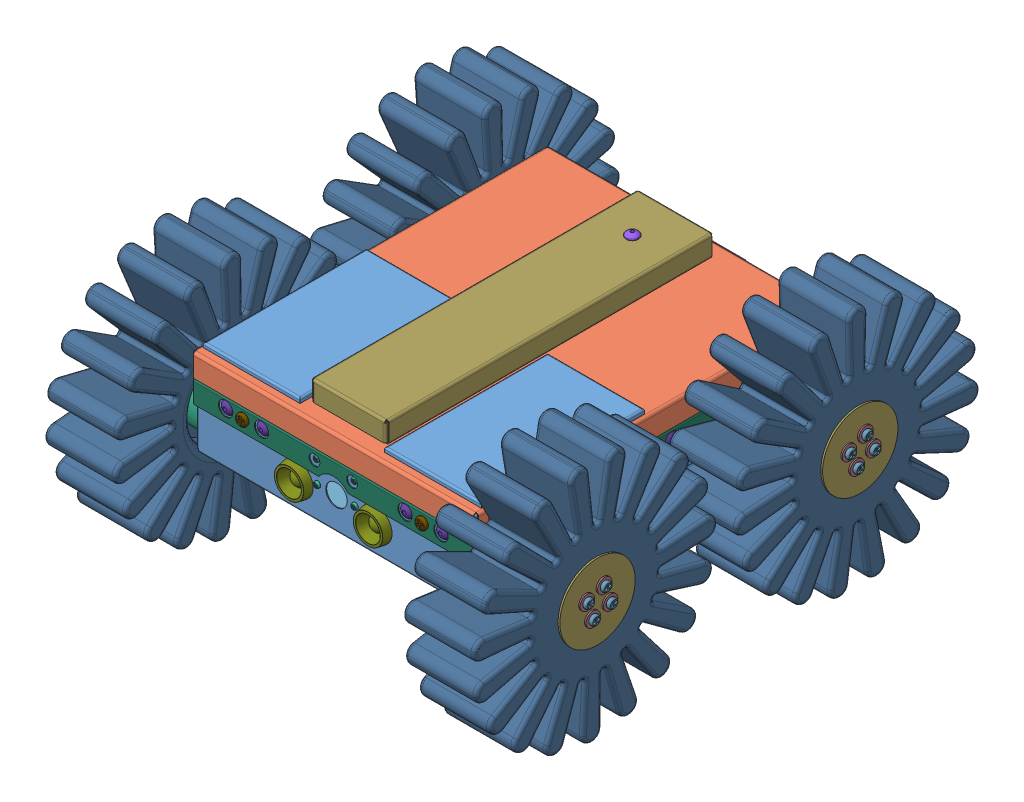
SolidWorks assembly GB0814, configuration Default. Lengths in mm.
Overall size (247.76 181.13 312.99).
487 component instances, 71 part files, 459 mates.
Components (placement in the parent):
- case.bottom-1: case.bottom [Default<As Machined>] at origin size (156 42.5 195.44)
- SM4315R-1: SM4315R [Default] at (47.1812 21 161.9111) x (0 -1 0) z (0 0 -1) size (20.32 45.78 53.29)
- SM4315R-2: SM4315R [Default] at (47.1812 21 17.796) x (0 1 0) z (0 0 1) size (20.32 45.78 53.29)
- SM4315R-3: SM4315R [Default] at (107.8188 21 17.796) x (0 -1 0) z (0 0 1) size (20.32 45.78 53.29)
- SM4315R-4: SM4315R [Default] at (107.8188 21 161.9111) x (0 1 0) z (0 0 -1) size (20.32 45.78 53.29)
- raspberrypi_b_+_(assembly)-1: raspberrypi_b_+_(assembly) [Valor predeterminado] at (78.9157 12.4 7.5062) x (0 0 -1) z (0 1 0) size (88.51 58.54 18.92)
  - raspberry_pi_B+_(bar_180_2x20)-1: raspberry_pi_B+_(bar_180_2x20) [Default] at (-150.8088 26.71 4.1) x (0 1 0) z (-1 0 0) size (5.08 11.6 50.8)
  - raspberry_pi_B+_(QFN64)-1: raspberry_pi_B+_(QFN64) [Default] at (-101.7896 6.9461 1.6) x (0 -1 0) z (-1 0 0) size (9.04 0.9 9.04)
  - raspberry_pi_B+_(168_FBGA_12x12)-1: raspberry_pi_B+_(168_FBGA_12x12) [Valor predeterminado] at (-129.6291 3.2481 1.87) size (12 12 0.71)
  - raspberry_pi_B+_(USB_x2)-1: raspberry_pi_B+_(USB_x2) [Valor predeterminado] at (-81.197 116.594 21.0675) x (0 1 0) z (1 0 0) size (14.7 17.85 17.4)
    - raspberry_pi_B+_(USB_x2_part1)-1: raspberry_pi_B+_(USB_x2_part1) [По умолчанию] at (-114.6616 -10.9375 -4.85) x (0 0 1) z (-1 0 0) size (17.4 6.35 14.7)
    - raspberry_pi_B+_(USB_x2_part2)-1: raspberry_pi_B+_(USB_x2_part2) [По умолчанию] at (-114.6616 -19.4375 -4.85) x (0 0 1) z (-1 0 0) size (17.4 11.5 14.7)
  - raspberry_pi_B+_(micro_USB)-1: raspberry_pi_B+_(micro_USB) [Default] at (-134.0345 -42.9478 -3.6369) x (1 0 0) z (0 -1 0) size (7.97 2.92 5.43)
    - raspberry_pi_B+_(micro_USB_cover)-1: raspberry_pi_B+_(micro_USB_cover) [Default] at (-14.4796 6.4719 -16.0085) size (7.97 2.92 5.43)
    - raspberry_pi_B+_(micro_USB_contacts)-1: raspberry_pi_B+_(micro_USB_contacts) [Default] at (-14.4796 6.4719 -20.7085) size (6.9 2.16 4.2)
  - raspberry_pi_B+_(HDMI_socket)-1: raspberry_pi_B+_(HDMI_socket) [Default] at (-127.1025 -18.8313 5.025) x (1 0 0) z (0 -1 0) size (16.2 8 9.9)
    - raspberry_pi__HDMI_socket_cover-1: raspberry_pi__HDMI_socket_cover [Default] at (-20 0 0) size (16.2 8 9)
    - raspberry_pi__HDMI_socket_inside-1: raspberry_pi__HDMI_socket_inside [Default] at (-20 0 0) size (15 6.1 7.6)
    - raspberry_pi__HDMI_socket_large_pin-1: raspberry_pi__HDMI_socket_large_pin [Valor predeterminado] at (-201.7661 0.45 76.5103) x (0 0 -1) z (0 -1 0) size (7.55 0.65 3.84)
    - raspberry_pi__HDMI_socket_small_pin-1: raspberry_pi__HDMI_socket_small_pin [Valor predeterminado] at (-202.2661 -0.25 76.5103) x (0 0 -1) z (0 -1 0) size (7.55 0.65 3.08)
    - raspberry_pi__HDMI_socket_large_pin-2: raspberry_pi__HDMI_socket_large_pin [Valor predeterminado] at (-202.7661 0.45 76.5103) x (0 0 -1) z (0 -1 0) size (7.55 0.65 3.84)
    - raspberry_pi__HDMI_socket_large_pin-3: raspberry_pi__HDMI_socket_large_pin [Valor predeterminado] at (-203.7661 0.45 76.5103) x (0 0 -1) z (0 -1 0) size (7.55 0.65 3.84)
    - raspberry_pi__HDMI_socket_large_pin-4: raspberry_pi__HDMI_socket_large_pin [Valor predeterminado] at (-204.7661 0.45 76.5103) x (0 0 -1) z (0 -1 0) size (7.55 0.65 3.84)
    - raspberry_pi__HDMI_socket_large_pin-5: raspberry_pi__HDMI_socket_large_pin [Valor predeterminado] at (-205.7661 0.45 76.5103) x (0 0 -1) z (0 -1 0) size (7.55 0.65 3.84)
    - raspberry_pi__HDMI_socket_large_pin-6: raspberry_pi__HDMI_socket_large_pin [Valor predeterminado] at (-206.7661 0.45 76.5103) x (0 0 -1) z (0 -1 0) size (7.55 0.65 3.84)
    - raspberry_pi__HDMI_socket_large_pin-7: raspberry_pi__HDMI_socket_large_pin [Valor predeterminado] at (-207.7661 0.45 76.5103) x (0 0 -1) z (0 -1 0) size (7.55 0.65 3.84)
    - raspberry_pi__HDMI_socket_large_pin-8: raspberry_pi__HDMI_socket_large_pin [Valor predeterminado] at (-208.7661 0.45 76.5103) x (0 0 -1) z (0 -1 0) size (7.55 0.65 3.84)
    - raspberry_pi__HDMI_socket_large_pin-9: raspberry_pi__HDMI_socket_large_pin [Valor predeterminado] at (-209.7661 0.45 76.5103) x (0 0 -1) z (0 -1 0) size (7.55 0.65 3.84)
    - raspberry_pi__HDMI_socket_large_pin-10: raspberry_pi__HDMI_socket_large_pin [Valor predeterminado] at (-210.7661 0.45 76.5103) x (0 0 -1) z (0 -1 0) size (7.55 0.65 3.84)
    - raspberry_pi__HDMI_socket_small_pin-2: raspberry_pi__HDMI_socket_small_pin [Valor predeterminado] at (-203.2661 -0.25 76.5103) x (0 0 -1) z (0 -1 0) size (7.55 0.65 3.08)
    - raspberry_pi__HDMI_socket_small_pin-3: raspberry_pi__HDMI_socket_small_pin [Valor predeterminado] at (-204.2661 -0.25 76.5103) x (0 0 -1) z (0 -1 0) size (7.55 0.65 3.08)
    - raspberry_pi__HDMI_socket_small_pin-4: raspberry_pi__HDMI_socket_small_pin [Valor predeterminado] at (-205.2661 -0.25 76.5103) x (0 0 -1) z (0 -1 0) size (7.55 0.65 3.08)
    - raspberry_pi__HDMI_socket_small_pin-5: raspberry_pi__HDMI_socket_small_pin [Valor predeterminado] at (-206.2661 -0.25 76.5103) x (0 0 -1) z (0 -1 0) size (7.55 0.65 3.08)
    - raspberry_pi__HDMI_socket_small_pin-6: raspberry_pi__HDMI_socket_small_pin [Valor predeterminado] at (-207.2661 -0.25 76.5103) x (0 0 -1) z (0 -1 0) size (7.55 0.65 3.08)
    - raspberry_pi__HDMI_socket_small_pin-7: raspberry_pi__HDMI_socket_small_pin [Valor predeterminado] at (-208.2661 -0.25 76.5103) x (0 0 -1) z (0 -1 0) size (7.55 0.65 3.08)
    - raspberry_pi__HDMI_socket_small_pin-8: raspberry_pi__HDMI_socket_small_pin [Valor predeterminado] at (-209.2661 -0.25 76.5103) x (0 0 -1) z (0 -1 0) size (7.55 0.65 3.08)
    - raspberry_pi__HDMI_socket_small_pin-9: raspberry_pi__HDMI_socket_small_pin [Valor predeterminado] at (-210.2661 -0.25 76.5103) x (0 0 -1) z (0 -1 0) size (7.55 0.65 3.08)
  - raspberry_pi_B+_(RJ45)-1: raspberry_pi_B+_(RJ45) [Default] at (-72.0064 -24.7094 15.1) x (0 1 0) z (1 0 0) size (15.88 16.5 21.4)
  - raspberry_pi_B+_(15_pin_FFC_Connector)-1: raspberry_pi_B+_(15_pin_FFC_Connector) [Valor predeterminado] at (-55.1145 1.0268 -17.4242) x (1 0 0) z (0 -1 0) size (4.85 6 22.4)
    - raspberry_pi__15_pin_FFC_Connector_body-1: raspberry_pi__15_pin_FFC_Connector_body [Valor predeterminado] at (-100.5372 19.1242 0) size (2.9 5.7 20.6)
    - raspberry_pi__15_pin_FFC_Connector_locker-1: raspberry_pi__15_pin_FFC_Connector_locker [Valor predeterminado] at (-101.0372 23.8242 0) size (4 5.4 22.4)
    - raspberry_pi__15_pin_FFC_Connector_pins-1: raspberry_pi__15_pin_FFC_Connector_pins [Valor predeterminado] at (-100.5372 19.1242 7.15) x (-1 0 0) z (0 0 -1) size (4.3 4.71 0.3)
    - raspberry_pi__15_pin_FFC_Connector_pins-2: raspberry_pi__15_pin_FFC_Connector_pins [Valor predeterminado] at (-100.5372 19.1242 6.15) x (-1 0 0) z (0 0 -1) size (4.3 4.71 0.3)
    - raspberry_pi__15_pin_FFC_Connector_pins-3: raspberry_pi__15_pin_FFC_Connector_pins [Valor predeterminado] at (-100.5372 19.1242 5.15) x (-1 0 0) z (0 0 -1) size (4.3 4.71 0.3)
    - raspberry_pi__15_pin_FFC_Connector_pins-4: raspberry_pi__15_pin_FFC_Connector_pins [Valor predeterminado] at (-100.5372 19.1242 4.15) x (-1 0 0) z (0 0 -1) size (4.3 4.71 0.3)
    - raspberry_pi__15_pin_FFC_Connector_pins-5: raspberry_pi__15_pin_FFC_Connector_pins [Valor predeterminado] at (-100.5372 19.1242 3.15) x (-1 0 0) z (0 0 -1) size (4.3 4.71 0.3)
    - raspberry_pi__15_pin_FFC_Connector_pins-6: raspberry_pi__15_pin_FFC_Connector_pins [Valor predeterminado] at (-100.5372 19.1242 2.15) x (-1 0 0) z (0 0 -1) size (4.3 4.71 0.3)
    - raspberry_pi__15_pin_FFC_Connector_pins-7: raspberry_pi__15_pin_FFC_Connector_pins [Valor predeterminado] at (-100.5372 19.1242 1.15) x (-1 0 0) z (0 0 -1) size (4.3 4.71 0.3)
    - raspberry_pi__15_pin_FFC_Connector_pins-8: raspberry_pi__15_pin_FFC_Connector_pins [Valor predeterminado] at (-100.5372 19.1242 0.15) x (-1 0 0) z (0 0 -1) size (4.3 4.71 0.3)
    - raspberry_pi__15_pin_FFC_Connector_pins-9: raspberry_pi__15_pin_FFC_Connector_pins [Valor predeterminado] at (-100.5372 19.1242 -0.85) x (-1 0 0) z (0 0 -1) size (4.3 4.71 0.3)
    - raspberry_pi__15_pin_FFC_Connector_pins-10: raspberry_pi__15_pin_FFC_Connector_pins [Valor predeterminado] at (-100.5372 19.1242 -1.85) x (-1 0 0) z (0 0 -1) size (4.3 4.71 0.3)
    - raspberry_pi__15_pin_FFC_Connector_pins-11: raspberry_pi__15_pin_FFC_Connector_pins [Valor predeterminado] at (-100.5372 19.1242 -2.85) x (-1 0 0) z (0 0 -1) size (4.3 4.71 0.3)
    - raspberry_pi__15_pin_FFC_Connector_pins-12: raspberry_pi__15_pin_FFC_Connector_pins [Valor predeterminado] at (-100.5372 19.1242 -3.85) x (-1 0 0) z (0 0 -1) size (4.3 4.71 0.3)
    - raspberry_pi__15_pin_FFC_Connector_pins-13: raspberry_pi__15_pin_FFC_Connector_pins [Valor predeterminado] at (-100.5372 19.1242 -4.85) x (-1 0 0) z (0 0 -1) size (4.3 4.71 0.3)
    - raspberry_pi__15_pin_FFC_Connector_pins-14: raspberry_pi__15_pin_FFC_Connector_pins [Valor predeterminado] at (-100.5372 19.1242 -5.85) x (-1 0 0) z (0 0 -1) size (4.3 4.71 0.3)
    - raspberry_pi__15_pin_FFC_Connector_pins-15: raspberry_pi__15_pin_FFC_Connector_pins [Valor predeterminado] at (-100.5372 19.1242 -6.85) x (-1 0 0) z (0 0 -1) size (4.3 4.71 0.3)
  - raspberry_pi_B+_(15_pin_FFC_Connector)-2: raspberry_pi_B+_(15_pin_FFC_Connector) [Valor predeterminado] at (-214.5607 -15.5826 -17.4242) x (-1 0 0) z (0 1 0) size (4.85 6 22.4)
    - raspberry_pi__15_pin_FFC_Connector_body-1: raspberry_pi__15_pin_FFC_Connector_body [Valor predeterminado] at (-100.5372 19.1242 0) size (2.9 5.7 20.6)
    - raspberry_pi__15_pin_FFC_Connector_locker-1: raspberry_pi__15_pin_FFC_Connector_locker [Valor predeterminado] at (-101.0372 23.8242 0) size (4 5.4 22.4)
    - raspberry_pi__15_pin_FFC_Connector_pins-1: raspberry_pi__15_pin_FFC_Connector_pins [Valor predeterminado] at (-100.5372 19.1242 7.15) x (-1 0 0) z (0 0 -1) size (4.3 4.71 0.3)
    - raspberry_pi__15_pin_FFC_Connector_pins-2: raspberry_pi__15_pin_FFC_Connector_pins [Valor predeterminado] at (-100.5372 19.1242 6.15) x (-1 0 0) z (0 0 -1) size (4.3 4.71 0.3)
    - raspberry_pi__15_pin_FFC_Connector_pins-3: raspberry_pi__15_pin_FFC_Connector_pins [Valor predeterminado] at (-100.5372 19.1242 5.15) x (-1 0 0) z (0 0 -1) size (4.3 4.71 0.3)
    - raspberry_pi__15_pin_FFC_Connector_pins-4: raspberry_pi__15_pin_FFC_Connector_pins [Valor predeterminado] at (-100.5372 19.1242 4.15) x (-1 0 0) z (0 0 -1) size (4.3 4.71 0.3)
    - raspberry_pi__15_pin_FFC_Connector_pins-5: raspberry_pi__15_pin_FFC_Connector_pins [Valor predeterminado] at (-100.5372 19.1242 3.15) x (-1 0 0) z (0 0 -1) size (4.3 4.71 0.3)
    - raspberry_pi__15_pin_FFC_Connector_pins-6: raspberry_pi__15_pin_FFC_Connector_pins [Valor predeterminado] at (-100.5372 19.1242 2.15) x (-1 0 0) z (0 0 -1) size (4.3 4.71 0.3)
    - raspberry_pi__15_pin_FFC_Connector_pins-7: raspberry_pi__15_pin_FFC_Connector_pins [Valor predeterminado] at (-100.5372 19.1242 1.15) x (-1 0 0) z (0 0 -1) size (4.3 4.71 0.3)
    - raspberry_pi__15_pin_FFC_Connector_pins-8: raspberry_pi__15_pin_FFC_Connector_pins [Valor predeterminado] at (-100.5372 19.1242 0.15) x (-1 0 0) z (0 0 -1) size (4.3 4.71 0.3)
    - raspberry_pi__15_pin_FFC_Connector_pins-9: raspberry_pi__15_pin_FFC_Connector_pins [Valor predeterminado] at (-100.5372 19.1242 -0.85) x (-1 0 0) z (0 0 -1) size (4.3 4.71 0.3)
    - raspberry_pi__15_pin_FFC_Connector_pins-10: raspberry_pi__15_pin_FFC_Connector_pins [Valor predeterminado] at (-100.5372 19.1242 -1.85) x (-1 0 0) z (0 0 -1) size (4.3 4.71 0.3)
    - raspberry_pi__15_pin_FFC_Connector_pins-11: raspberry_pi__15_pin_FFC_Connector_pins [Valor predeterminado] at (-100.5372 19.1242 -2.85) x (-1 0 0) z (0 0 -1) size (4.3 4.71 0.3)
    - raspberry_pi__15_pin_FFC_Connector_pins-12: raspberry_pi__15_pin_FFC_Connector_pins [Valor predeterminado] at (-100.5372 19.1242 -3.85) x (-1 0 0) z (0 0 -1) size (4.3 4.71 0.3)
    - raspberry_pi__15_pin_FFC_Connector_pins-13: raspberry_pi__15_pin_FFC_Connector_pins [Valor predeterminado] at (-100.5372 19.1242 -4.85) x (-1 0 0) z (0 0 -1) size (4.3 4.71 0.3)
    - raspberry_pi__15_pin_FFC_Connector_pins-14: raspberry_pi__15_pin_FFC_Connector_pins [Valor predeterminado] at (-100.5372 19.1242 -5.85) x (-1 0 0) z (0 0 -1) size (4.3 4.71 0.3)
    - raspberry_pi__15_pin_FFC_Connector_pins-15: raspberry_pi__15_pin_FFC_Connector_pins [Valor predeterminado] at (-100.5372 19.1242 -6.85) x (-1 0 0) z (0 0 -1) size (4.3 4.71 0.3)
  - raspberry_pi_B+_(CI_Board)-1: raspberry_pi_B+_(CI_Board) [Default] at (-116.6004 0.9483 0) size (85 56 1.6)
  - raspberry_pi_B+_(USB_x2)-2: raspberry_pi_B+_(USB_x2) [Valor predeterminado] at (-81.2313 134.607 21.0675) x (0 1 0) z (1 0 0) size (14.7 17.85 17.4)
    - raspberry_pi_B+_(USB_x2_part1)-1: raspberry_pi_B+_(USB_x2_part1) [По умолчанию] at (-114.6616 -10.9375 -4.85) x (0 0 1) z (-1 0 0) size (17.4 6.35 14.7)
    - raspberry_pi_B+_(USB_x2_part2)-1: raspberry_pi_B+_(USB_x2_part2) [По умолчанию] at (-114.6616 -19.4375 -4.85) x (0 0 1) z (-1 0 0) size (17.4 11.5 14.7)
  - raspberry_pi_B+_(microsd_slot2)-1: raspberry_pi_B+_(microsd_slot2) [Default] at (-159.8159 1.7594 -0.765) x (0 1 0) z (-1 0 0) size (14.6 1.73 16)
  - raspberry_pi_B+_(microsd2)-1: raspberry_pi_B+_(microsd2) [Default] at (-152.7882 0.8694 -0.87) x (1 0 0) z (0 1 0) size (15 1 11)
  - raspberry_pi_B+_(audio_video2)-1: raspberry_pi_B+_(audio_video2) [Default] at (-105.6017 -27.0888 1.6) x (0 1 0) z (1 0 0) size (19 5.8 7.5)
- SM4315R.horn-1: SM4315R.horn [Default] at (4.9 21 16.636) x (-1 0 0) z (0 -1 0) size (5.4 20.9 20.9)
- SM4315R.horn-2: SM4315R.horn [Default] at (4.9 21 163.0711) x (-1 0 0) z (0 -0.955985 -0.293416) size (5.4 20.9 20.9)
- SM4315R.horn-3: SM4315R.horn [Default] at (150.1 21 16.636) x (1 0 0) z (0 0.339591 0.940573) size (5.4 20.9 20.9)
- SM4315R.horn-4: SM4315R.horn [Default] at (150.1 21 163.0711) x (1 0 0) z (0 0.895983 -0.444088) size (5.4 20.9 20.9)
- accumulator-1: accumulator [Default] at (76.0287 1 180.3909) x (-1 0 0) z (0 0 -1) size (55 6 90)
- accumulator-2: accumulator [Default] at (133.5703 1 180.9066) x (-1 0 0) z (0 0 -1) size (55 6 90)
- accumulator-3: accumulator [Default] at (21.0287 1 -0.1494) size (55 6 90)
- accumulator-4: accumulator [Default] at (78.5703 1 -0.1494) size (55 6 90)
- flange-1: flange [Default] at (-0.5 21.0015 16.8638) x (0 0.99991 -0.013396) z (0 0.013396 0.99991) size (40 15 40)
- wheel.hub-1: wheel.hub [Default] at (-0.5 21 16.636) x (0 0.999959 0.009009) z (0 -0.009009 0.999959) size (26 16 26)
- pin.2.54.holder-1: pin.2.54.holder [Default] at (52.2307 16.5 112.57) size (2.5 14.25 2.5)
- self.stop.nut.m3-1: self.stop.nut.m3 [Default] at (0 21.2293 33.8623) x (0 -1 0) z (0 0 1) size (6.78 4 6.27)
- self.stop.nut.m3-2: self.stop.nut.m3 [Default] at (0 38 16.636) x (0 -1 0) z (0 0 1) size (6.78 4 6.27)
- self.stop.nut.m3-3: self.stop.nut.m3 [Default] at (0 20.7738 -0.1347) x (0 -1 0) z (0 0 1) size (6.78 4 6.27)
- self.stop.nut.m3-4: self.stop.nut.m3 [Default] at (0 4.0031 17.0915) x (0 -1 0) z (0 0 1) size (6.78 4 6.27)
- ball.4mm-1: ball.4mm [Default] at (-2.5 12.5205 25.8201) size (4 4 4)
- ball.4mm-2: ball.4mm [Default] at (-2.5 15.962 28.0758) x (1 0 0) z (0 0.324699 0.945817) size (4 4 4)
- ball.4mm-3: ball.4mm [Default] at (-2.5 19.9494 29.0918) x (1 0 0) z (0 0.614213 0.789141) size (4 4 4)
- ball.4mm-4: ball.4mm [Default] at (-2.5 24.0508 28.758) x (1 0 0) z (0 0.837166 0.546948) size (4 4 4)
- ball.4mm-5: ball.4mm [Default] at (-2.5 27.8215 27.1107) x (1 0 0) z (0 0.9694 0.245485) size (4 4 4)
- ball.4mm-6: ball.4mm [Default] at (-2.5 30.853 24.3282) x (1 0 0) z (0 0.996584 -0.082579) size (4 4 4)
- ball.4mm-7: ball.4mm [Default] at (-2.5 32.8167 20.7122) x (1 0 0) z (0 0.915773 -0.401695) size (4 4 4)
- ball.4mm-8: ball.4mm [Default] at (-2.5 33.5 16.6544) x (1 0 0) z (0 0.735724 -0.677282) size (4 4 4)
- ball.4mm-9: ball.4mm [Default] at (-2.5 32.8287 12.5947) x (1 0 0) z (0 0.475947 -0.879474) size (4 4 4)
- ball.4mm-10: ball.4mm [Default] at (-2.5 30.8755 8.9729) x (1 0 0) z (0 0.164595 -0.986361) size (4 4 4)
- ball.4mm-11: ball.4mm [Default] at (-2.5 27.8522 6.1815) x (1 0 0) z (0 -0.164595 -0.986361) size (4 4 4)
- ball.4mm-12: ball.4mm [Default] at (-2.5 24.0864 4.5231) x (1 0 0) z (0 -0.475947 -0.879474) size (4 4 4)
- ball.4mm-13: ball.4mm [Default] at (-2.5 19.9861 4.1772) x (1 0 0) z (0 -0.735724 -0.677282) size (4 4 4)
- ball.4mm-14: ball.4mm [Default] at (-2.5 15.9956 5.1815) x (1 0 0) z (0 -0.915773 -0.401695) size (4 4 4)
- ball.4mm-15: ball.4mm [Default] at (-2.5 12.5475 7.4271) x (1 0 0) z (0 -0.996584 -0.082579) size (4 4 4)
- ball.4mm-16: ball.4mm [Default] at (-2.5 10.0153 10.6705) x (1 0 0) z (0 -0.9694 0.245485) size (4 4 4)
- ball.4mm-17: ball.4mm [Default] at (-2.5 8.6735 14.5605) x (1 0 0) z (0 -0.837166 0.546948) size (4 4 4)
- ball.4mm-18: ball.4mm [Default] at (-2.5 8.6675 18.6753) x (1 0 0) z (0 -0.614213 0.789141) size (4 4 4)
- m3.screw.18mm-2: m3.screw.18mm [Default] at (-15.5 38 16.636) x (0 -1 0) z (0 0 1) size (5 20.25 5)
- m3.screw.18mm-3: m3.screw.18mm [Default] at (-15.5 4.0031 17.0915) x (0 -1 0) z (0 0 1) size (5 20.25 5)
- m3.screw.18mm-4: m3.screw.18mm [Default] at (-15.5 20.7738 -0.1347) x (0 -1 0) z (0 0 1) size (5 20.25 5)
- m3.screw.18mm-5: m3.screw.18mm [Default] at (-15.5 21.2293 33.8623) x (0 -1 0) z (0 0 1) size (5 20.25 5)
- m3.screw.30mm-6: m3.screw.30mm [Default] at (-16.5 21 16.636) x (0 -1 0) z (0 0 1) size (5 32.25 5)
- ball.4mm-19: ball.4mm [Default] at (-10.5 16.8546 5.0717) size (4 4 4)
- ball.4mm-20: ball.4mm [Default] at (-10.5 13.3243 7.0443) x (1 0 0) z (0 0.324699 0.945817) size (4 4 4)
- ball.4mm-21: ball.4mm [Default] at (-10.5 10.6257 10.0563) x (1 0 0) z (0 0.614213 0.789141) size (4 4 4)
- ball.4mm-22: ball.4mm [Default] at (-10.5 9.0514 13.7814) x (1 0 0) z (0 0.837166 0.546948) size (4 4 4)
- ball.4mm-23: ball.4mm [Default] at (-10.5 8.7719 17.8157) x (1 0 0) z (0 0.9694 0.245485) size (4 4 4)
- ball.4mm-24: ball.4mm [Default] at (-10.5 9.8175 21.7223) x (1 0 0) z (0 0.996584 -0.082579) size (4 4 4)
- ball.4mm-25: ball.4mm [Default] at (-10.5 12.0749 25.0776) x (1 0 0) z (0 0.915773 -0.401695) size (4 4 4)
- ball.4mm-26: ball.4mm [Default] at (-10.5 15.2995 27.5182) x (1 0 0) z (0 0.735724 -0.677282) size (4 4 4)
- ball.4mm-27: ball.4mm [Default] at (-10.5 19.1418 28.7796) x (1 0 0) z (0 0.475947 -0.879474) size (4 4 4)
- ball.4mm-28: ball.4mm [Default] at (-10.5 23.1855 28.725) x (1 0 0) z (0 0.164595 -0.986361) size (4 4 4)
- ball.4mm-29: ball.4mm [Default] at (-10.5 26.9923 27.3603) x (1 0 0) z (0 -0.164595 -0.986361) size (4 4 4)
- ball.4mm-30: ball.4mm [Default] at (-10.5 30.1498 24.8336) x (1 0 0) z (0 -0.475947 -0.879474) size (4 4 4)
- ball.4mm-31: ball.4mm [Default] at (-10.5 32.3158 21.4185) x (1 0 0) z (0 -0.735724 -0.677282) size (4 4 4)
- ball.4mm-32: ball.4mm [Default] at (-10.5 33.2555 17.4851) x (1 0 0) z (0 -0.915773 -0.401695) size (4 4 4)
- ball.4mm-33: ball.4mm [Default] at (-10.5 32.8672 13.4597) x (1 0 0) z (0 -0.996584 -0.082579) size (4 4 4)
- ball.4mm-34: ball.4mm [Default] at (-10.5 31.1928 9.7786) x (1 0 0) z (0 -0.9694 0.245485) size (4 4 4)
- ball.4mm-35: ball.4mm [Default] at (-10.5 28.4139 6.8405) x (1 0 0) z (0 -0.837166 0.546948) size (4 4 4)
- ball.4mm-36: ball.4mm [Default] at (-10.5 24.8316 4.964) x (1 0 0) z (0 -0.614213 0.789141) size (4 4 4)
- wheel.hub-2: wheel.hub [Default] at (-0.5 21 163.0711) x (0 -0.293416 0.955985) z (0 -0.955985 -0.293416) size (26 16 26)
- m3.screw.30mm-7: m3.screw.30mm [Default] at (-16.5 21 163.0711) x (0 -1 0) z (0 0 1) size (5 32.25 5)
- ball.4mm-37: ball.4mm [Default] at (-2.5 28.5181 173.0574) size (4 4 4)
- ball.4mm-38: ball.4mm [Default] at (-2.5 31.3533 170.0752) x (1 0 0) z (0 0.324699 0.945817) size (4 4 4)
- ball.4mm-39: ball.4mm [Default] at (-2.5 33.0666 166.334) x (1 0 0) z (0 0.614213 0.789141) size (4 4 4)
- ball.4mm-40: ball.4mm [Default] at (-2.5 33.4723 162.2392) x (1 0 0) z (0 0.837166 0.546948) size (4 4 4)
- ball.4mm-41: ball.4mm [Default] at (-2.5 32.5264 158.2345) x (1 0 0) z (0 0.9694 0.245485) size (4 4 4)
- ball.4mm-42: ball.4mm [Default] at (-2.5 30.3314 154.7539) x (1 0 0) z (0 0.996584 -0.082579) size (4 4 4)
- ball.4mm-43: ball.4mm [Default] at (-2.5 27.1253 152.1747) x (1 0 0) z (0 0.915773 -0.401695) size (4 4 4)
- ball.4mm-44: ball.4mm [Default] at (-2.5 23.2553 150.7762) x (1 0 0) z (0 0.735724 -0.677282) size (4 4 4)
- ball.4mm-45: ball.4mm [Default] at (-2.5 19.141 150.7101) x (1 0 0) z (0 0.475947 -0.879474) size (4 4 4)
- ball.4mm-46: ball.4mm [Default] at (-2.5 15.2281 151.9834) x (1 0 0) z (0 0.164595 -0.986361) size (4 4 4)
- ball.4mm-47: ball.4mm [Default] at (-2.5 11.9407 154.4583) x (1 0 0) z (0 -0.164595 -0.986361) size (4 4 4)
- ball.4mm-48: ball.4mm [Default] at (-2.5 9.635 157.8665) x (1 0 0) z (0 -0.475947 -0.879474) size (4 4 4)
- ball.4mm-49: ball.4mm [Default] at (-2.5 8.5609 161.8387) x (1 0 0) z (0 -0.735724 -0.677282) size (4 4 4)
- ball.4mm-50: ball.4mm [Default] at (-2.5 8.8347 165.9445) x (1 0 0) z (0 -0.915773 -0.401695) size (4 4 4)
- ball.4mm-51: ball.4mm [Default] at (-2.5 10.4269 169.7389) x (1 0 0) z (0 -0.996584 -0.082579) size (4 4 4)
- ball.4mm-52: ball.4mm [Default] at (-2.5 13.1648 172.8107) x (1 0 0) z (0 -0.9694 0.245485) size (4 4 4)
- ball.4mm-53: ball.4mm [Default] at (-2.5 16.7518 174.827) x (1 0 0) z (0 -0.837166 0.546948) size (4 4 4)
- ball.4mm-54: ball.4mm [Default] at (-2.5 20.7991 175.5695) x (1 0 0) z (0 -0.614213 0.789141) size (4 4 4)
- ball.4mm-55: ball.4mm [Default] at (-10.5 14.3874 173.6788) size (4 4 4)
- ball.4mm-56: ball.4mm [Default] at (-10.5 18.19 175.2511) x (1 0 0) z (0 0.324699 0.945817) size (4 4 4)
- ball.4mm-57: ball.4mm [Default] at (-10.5 22.2971 175.5036) x (1 0 0) z (0 0.614213 0.789141) size (4 4 4)
- ball.4mm-58: ball.4mm [Default] at (-10.5 26.2637 174.4088) x (1 0 0) z (0 0.837166 0.546948) size (4 4 4)
- ball.4mm-59: ball.4mm [Default] at (-10.5 29.6598 172.0854) x (1 0 0) z (0 0.9694 0.245485) size (4 4 4)
- ball.4mm-60: ball.4mm [Default] at (-10.5 32.1176 168.7851) x (1 0 0) z (0 0.996584 -0.082579) size (4 4 4)
- ball.4mm-61: ball.4mm [Default] at (-10.5 33.3705 164.8656) x (1 0 0) z (0 0.915773 -0.401695) size (4 4 4)
- ball.4mm-62: ball.4mm [Default] at (-10.5 33.2829 160.7517) x (1 0 0) z (0 0.735724 -0.677282) size (4 4 4)
- ball.4mm-63: ball.4mm [Default] at (-10.5 31.8643 156.8891) x (1 0 0) z (0 0.475947 -0.879474) size (4 4 4)
- ball.4mm-64: ball.4mm [Default] at (-10.5 29.2684 153.6964) x (1 0 0) z (0 0.164595 -0.986361) size (4 4 4)
- ball.4mm-65: ball.4mm [Default] at (-10.5 25.7764 151.5196) x (1 0 0) z (0 -0.164595 -0.986361) size (4 4 4)
- ball.4mm-66: ball.4mm [Default] at (-10.5 21.7669 150.5946) x (1 0 0) z (0 -0.475947 -0.879474) size (4 4 4)
- ball.4mm-67: ball.4mm [Default] at (-10.5 17.6742 151.0216) x (1 0 0) z (0 -0.735724 -0.677282) size (4 4 4)
- ball.4mm-68: ball.4mm [Default] at (-10.5 13.942 152.7544) x (1 0 0) z (0 -0.915773 -0.401695) size (4 4 4)
- ball.4mm-69: ball.4mm [Default] at (-10.5 10.9746 155.6051) x (1 0 0) z (0 -0.996584 -0.082579) size (4 4 4)
- ball.4mm-70: ball.4mm [Default] at (-10.5 9.0936 159.2649) x (1 0 0) z (0 -0.9694 0.245485) size (4 4 4)
- ball.4mm-71: ball.4mm [Default] at (-10.5 8.5028 163.3371) x (1 0 0) z (0 -0.837166 0.546948) size (4 4 4)
- ball.4mm-72: ball.4mm [Default] at (-10.5 9.2663 167.3805) x (1 0 0) z (0 -0.614213 0.789141) size (4 4 4)
- flange-2: flange [Default] at (-0.5 21 163.0711) x (0 1 0) z (0 0 1) size (40 15 40)
- m3.screw.18mm-6: m3.screw.18mm [Default] at (-15.5 4 163.0711) x (0 -1 0) z (0 0 1) size (5 20.25 5)
- m3.screw.18mm-7: m3.screw.18mm [Default] at (-15.5 21 146.0711) x (0 -1 0) z (0 0 1) size (5 20.25 5)
- m3.screw.18mm-8: m3.screw.18mm [Default] at (-15.5 38 163.0711) x (0 -1 0) z (0 0 1) size (5 20.25 5)
- m3.screw.18mm-9: m3.screw.18mm [Default] at (-15.5 21 180.0711) x (0 -1 0) z (0 0 1) size (5 20.25 5)
- wheel.hub-3: wheel.hub [Default] at (155.5 21 163.0711) x (0 0.444088 0.895983) z (0 0.895983 -0.444088) size (26 16 26)
- self.stop.nut.m3-5: self.stop.nut.m3 [Default] at (0 38 163.0711) x (0 -1 0) z (0 0 1) size (6.78 4 6.27)
- self.stop.nut.m3-6: self.stop.nut.m3 [Default] at (0 21 180.0711) x (0 -1 0) z (0 0 1) size (6.78 4 6.27)
- self.stop.nut.m3-7: self.stop.nut.m3 [Default] at (0 21 146.0711) x (0 -1 0) z (0 0 1) size (6.78 4 6.27)
- self.stop.nut.m3-8: self.stop.nut.m3 [Default] at (0 4 163.0711) x (0 -1 0) z (0 0 1) size (6.78 4 6.27)
- m2.screw-1: m2.screw [Default] at (1.4 18.8918 170.0041) x (0 -0.781504 0.6239) z (-1 0 0) size (3.34 3.34 9.36)
- m2.screw-2: m2.screw [Default] at (1.4 23.1324 156.1217) x (0 0.492887 0.870093) z (-1 0 0) size (3.34 3.34 9.36)
- m2.screw-3: m2.screw [Default] at (1.4 27.944 165.1843) x (0 0.031188 0.999514) z (-1 0 0) size (3.34 3.34 9.36)
- m2.screw-4: m2.screw [Default] at (1.4 14.0879 160.948) x (0 -0.845824 0.533463) z (-1 0 0) size (3.34 3.34 9.36)
- m2.screw-5: m2.screw [Default] at (1.4 13.7636 16.6224) x (0 0 1) z (-1 0 0) size (3.34 3.34 9.36)
- m2.screw-6: m2.screw [Default] at (1.4 21.0136 9.3724) x (0 0 1) z (-1 0 0) size (3.34 3.34 9.36)
- m2.screw-7: m2.screw [Default] at (1.4 21.0136 23.8724) x (0 0 1) z (-1 0 0) size (3.34 3.34 9.36)
- m2.screw-8: m2.screw [Default] at (1.4 28.2636 16.6224) x (0 0 1) z (-1 0 0) size (3.34 3.34 9.36)
- ball.4mm-73: ball.4mm [Default] at (157.5 14.8528 152.1871) size (4 4 4)
- ball.4mm-74: ball.4mm [Default] at (157.5 18.7199 150.7808) x (1 0 0) z (0 -0.324699 0.945817) size (4 4 4)
- ball.4mm-75: ball.4mm [Default] at (157.5 22.8341 150.7064) x (1 0 0) z (0 -0.614213 0.789141) size (4 4 4)
- ball.4mm-76: ball.4mm [Default] at (157.5 26.7495 151.9718) x (1 0 0) z (0 -0.837166 0.546948) size (4 4 4)
- ball.4mm-77: ball.4mm [Default] at (157.5 30.0419 154.4401) x (1 0 0) z (0 -0.9694 0.245485) size (4 4 4)
- ball.4mm-78: ball.4mm [Default] at (157.5 32.3545 157.8436) x (1 0 0) z (0 -0.996584 -0.082579) size (4 4 4)
- ball.4mm-79: ball.4mm [Default] at (157.5 33.4366 161.8137) x (1 0 0) z (0 -0.915773 -0.401695) size (4 4 4)
- ball.4mm-80: ball.4mm [Default] at (157.5 33.171 165.9199) x (1 0 0) z (0 -0.735724 -0.677282) size (4 4 4)
- ball.4mm-81: ball.4mm [Default] at (157.5 31.5865 169.7175) x (1 0 0) z (0 -0.475947 -0.879474) size (4 4 4)
- ball.4mm-82: ball.4mm [Default] at (157.5 28.8548 172.7948) x (1 0 0) z (0 -0.164595 -0.986361) size (4 4 4)
- ball.4mm-83: ball.4mm [Default] at (157.5 25.2719 174.8184) x (1 0 0) z (0 0.164595 -0.986361) size (4 4 4)
- ball.4mm-84: ball.4mm [Default] at (157.5 21.2261 175.569) x (1 0 0) z (0 0.475947 -0.879474) size (4 4 4)
- ball.4mm-85: ball.4mm [Default] at (157.5 17.1558 174.9653) x (1 0 0) z (0 0.735724 -0.677282) size (4 4 4)
- ball.4mm-86: ball.4mm [Default] at (157.5 13.502 173.0726) x (1 0 0) z (0 0.915773 -0.401695) size (4 4 4)
- ball.4mm-87: ball.4mm [Default] at (157.5 10.6608 170.0961) x (1 0 0) z (0 0.996584 -0.082579) size (4 4 4)
- ball.4mm-88: ball.4mm [Default] at (157.5 8.94 166.3583) x (1 0 0) z (0 0.9694 0.245485) size (4 4 4)
- ball.4mm-89: ball.4mm [Default] at (157.5 8.5261 162.2643) x (1 0 0) z (0 0.837166 0.546948) size (4 4 4)
- ball.4mm-90: ball.4mm [Default] at (157.5 9.4639 158.2578) x (1 0 0) z (0 0.614213 0.789141) size (4 4 4)
- ball.4mm-91: ball.4mm [Default] at (157.5 11.6518 154.7728) x (1 0 0) z (0 0.324699 0.945817) size (4 4 4)
- ball.4mm-92: ball.4mm [Default] at (-2.5 9.9978 22.5692) x (1 0 0) z (0 -0.324699 0.945817) size (4 4 4)
- ball.4mm-93: ball.4mm [Default] at (-10.5 20.8341 4.3523) x (1 0 0) z (0 -0.324699 0.945817) size (4 4 4)
- ball.4mm-94: ball.4mm [Default] at (-2.5 24.8682 174.9575) x (1 0 0) z (0 -0.324699 0.945817) size (4 4 4)
- ball.4mm-95: ball.4mm [Default] at (-10.5 11.3014 170.9569) x (1 0 0) z (0 -0.324699 0.945817) size (4 4 4)
- ball.4mm-96: ball.4mm [Default] at (165.5 29.4044 172.3239) size (4 4 4)
- ball.4mm-97: ball.4mm [Default] at (165.5 25.9446 174.5515) x (1 0 0) z (0 -0.324699 0.945817) size (4 4 4)
- ball.4mm-98: ball.4mm [Default] at (165.5 21.949 175.535) x (1 0 0) z (0 -0.614213 0.789141) size (4 4 4)
- ball.4mm-99: ball.4mm [Default] at (165.5 17.8506 175.1678) x (1 0 0) z (0 -0.837166 0.546948) size (4 4 4)
- ball.4mm-100: ball.4mm [Default] at (165.5 14.0934 173.4898) x (1 0 0) z (0 -0.9694 0.245485) size (4 4 4)
- ball.4mm-101: ball.4mm [Default] at (165.5 11.0847 170.6827) x (1 0 0) z (0 -0.996584 -0.082579) size (4 4 4)
- ball.4mm-102: ball.4mm [Default] at (165.5 9.1504 167.0508) x (1 0 0) z (0 -0.915773 -0.401695) size (4 4 4)
- ball.4mm-103: ball.4mm [Default] at (165.5 8.5003 162.9876) x (1 0 0) z (0 -0.735724 -0.677282) size (4 4 4)
- ball.4mm-104: ball.4mm [Default] at (165.5 9.2046 158.9335) x (1 0 0) z (0 -0.475947 -0.879474) size (4 4 4)
- ball.4mm-105: ball.4mm [Default] at (165.5 11.1872 155.3277) x (1 0 0) z (0 -0.164595 -0.986361) size (4 4 4)
- ball.4mm-106: ball.4mm [Default] at (165.5 14.2332 152.5611) x (1 0 0) z (0 0.164595 -0.986361) size (4 4 4)
- ball.4mm-107: ball.4mm [Default] at (165.5 18.0124 150.9333) x (1 0 0) z (0 0.475947 -0.879474) size (4 4 4)
- ball.4mm-108: ball.4mm [Default] at (165.5 22.1154 150.6209) x (1 0 0) z (0 0.735724 -0.677282) size (4 4 4)
- ball.4mm-109: ball.4mm [Default] at (165.5 26.0975 151.6577) x (1 0 0) z (0 0.915773 -0.401695) size (4 4 4)
- ball.4mm-110: ball.4mm [Default] at (165.5 29.5272 153.9313) x (1 0 0) z (0 0.996584 -0.082579) size (4 4 4)
- ball.4mm-111: ball.4mm [Default] at (165.5 32.0329 157.1953) x (1 0 0) z (0 0.9694 0.245485) size (4 4 4)
- ball.4mm-112: ball.4mm [Default] at (165.5 33.343 161.096) x (1 0 0) z (0 0.837166 0.546948) size (4 4 4)
- ball.4mm-113: ball.4mm [Default] at (165.5 33.3155 165.2108) x (1 0 0) z (0 0.614213 0.789141) size (4 4 4)
- ball.4mm-114: ball.4mm [Default] at (165.5 31.9535 169.0937) x (1 0 0) z (0 0.324699 0.945817) size (4 4 4)
- flange-3: flange [Default] at (155.5 21 163.0711) x (0 -1 0) z (0 0 1) size (40 15 40)
- m3.screw.30mm-8: m3.screw.30mm [Default] at (171.5 21 163.0711) x (0 1 0) z (0 0 1) size (5 32.25 5)
- m3.screw.18mm-10: m3.screw.18mm [Default] at (170.5 38 163.0711) x (0 1 0) z (0 0 1) size (5 20.25 5)
- m3.screw.18mm-11: m3.screw.18mm [Default] at (170.5 21 180.0711) x (0 1 0) z (0 0 1) size (5 20.25 5)
- m3.screw.18mm-12: m3.screw.18mm [Default] at (170.5 21 146.0711) x (0 1 0) z (0 0 1) size (5 20.25 5)
- m3.screw.18mm-13: m3.screw.18mm [Default] at (170.5 4 163.0711) x (0 1 0) z (0 0 1) size (5 20.25 5)
- self.stop.nut.m3-9: self.stop.nut.m3 [Default] at (155 4 163.0711) x (0 1 0) z (0 0 1) size (6.78 4 6.27)
- self.stop.nut.m3-10: self.stop.nut.m3 [Default] at (155 21 180.0711) x (0 1 0) z (0 0 1) size (6.78 4 6.27)
- self.stop.nut.m3-11: self.stop.nut.m3 [Default] at (155 38 163.0711) x (0 1 0) z (0 0 1) size (6.78 4 6.27)
- self.stop.nut.m3-12: self.stop.nut.m3 [Default] at (155 21 146.0711) x (0 1 0) z (0 0 1) size (6.78 4 6.27)
- m2.screw-9: m2.screw [Default] at (153.6 24.2061 169.5534) x (0 0 1) z (1 0 0) size (3.34 3.34 9.36)
- m2.screw-10: m2.screw [Default] at (153.6 14.4933 166.3066) x (0 0.983087 -0.183139) z (1 0 0) size (3.34 3.34 9.36)
- m2.screw-11: m2.screw [Default] at (153.6 27.5095 159.865) x (0 0 -1) z (1 0 0) size (3.34 3.34 9.36)
- m2.screw-12: m2.screw [Default] at (153.6 17.7939 156.5888) x (0 0 -1) z (1 0 0) size (3.34 3.34 9.36)
- wheel.hub-4: wheel.hub [Default] at (155.5 21 16.636) x (0 -0.940573 0.339591) z (0 0.339591 0.940573) size (26 16 26)
- ball.4mm-115: ball.4mm [Default] at (157.5 31.533 9.9051) size (4 4 4)
- ball.4mm-116: ball.4mm [Default] at (165.5 16.1371 5.1207) size (4 4 4)
- ball.4mm-117: ball.4mm [Default] at (157.5 28.7768 6.8497) x (1 0 0) z (0 0.324699 0.945817) size (4 4 4)
- ball.4mm-118: ball.4mm [Default] at (157.5 25.1778 4.8549) x (1 0 0) z (0 0.614213 0.789141) size (4 4 4)
- ball.4mm-119: ball.4mm [Default] at (157.5 21.1261 4.1367) x (1 0 0) z (0 0.837166 0.546948) size (4 4 4)
- ball.4mm-120: ball.4mm [Default] at (157.5 17.0607 4.773) x (1 0 0) z (0 0.9694 0.245485) size (4 4 4)
- ball.4mm-121: ball.4mm [Default] at (157.5 13.4222 6.6948) x (1 0 0) z (0 0.996584 -0.082579) size (4 4 4)
- ball.4mm-122: ball.4mm [Default] at (157.5 10.6049 9.694) x (1 0 0) z (0 0.915773 -0.401695) size (4 4 4)
- ball.4mm-123: ball.4mm [Default] at (157.5 8.9141 13.4454) x (1 0 0) z (0 0.735724 -0.677282) size (4 4 4)
- ball.4mm-124: ball.4mm [Default] at (157.5 8.5329 17.5426) x (1 0 0) z (0 0.475947 -0.879474) size (4 4 4)
- ball.4mm-125: ball.4mm [Default] at (157.5 9.5028 21.5415) x (1 0 0) z (0 0.164595 -0.986361) size (4 4 4)
- ball.4mm-126: ball.4mm [Default] at (157.5 11.7185 25.0089) x (1 0 0) z (0 -0.164595 -0.986361) size (4 4 4)
- ball.4mm-127: ball.4mm [Default] at (157.5 14.9401 27.5689) x (1 0 0) z (0 -0.475947 -0.879474) size (4 4 4)
- ball.4mm-128: ball.4mm [Default] at (157.5 18.8183 28.9442) x (1 0 0) z (0 -0.735724 -0.677282) size (4 4 4)
- ball.4mm-129: ball.4mm [Default] at (157.5 22.933 28.9857) x (1 0 0) z (0 -0.915773 -0.401695) size (4 4 4)
- ball.4mm-130: ball.4mm [Default] at (157.5 26.8381 27.6889) x (1 0 0) z (0 -0.996584 -0.082579) size (4 4 4)
- ball.4mm-131: ball.4mm [Default] at (157.5 30.1107 25.1944) x (1 0 0) z (0 -0.9694 0.245485) size (4 4 4)
- ball.4mm-132: ball.4mm [Default] at (157.5 32.3959 21.7724) x (1 0 0) z (0 -0.837166 0.546948) size (4 4 4)
- ball.4mm-133: ball.4mm [Default] at (157.5 33.4463 17.7939) x (1 0 0) z (0 -0.614213 0.789141) size (4 4 4)
- ball.4mm-134: ball.4mm [Default] at (157.5 33.1478 13.6899) x (1 0 0) z (0 -0.324699 0.945817) size (4 4 4)
- ball.4mm-135: ball.4mm [Default] at (165.5 20.1396 4.1657) x (1 0 0) z (0 -0.324699 0.945817) size (4 4 4)
- ball.4mm-136: ball.4mm [Default] at (165.5 24.2353 4.562) x (1 0 0) z (0 -0.614213 0.789141) size (4 4 4)
- ball.4mm-137: ball.4mm [Default] at (165.5 27.9805 6.2667) x (1 0 0) z (0 -0.837166 0.546948) size (4 4 4)
- ball.4mm-138: ball.4mm [Default] at (165.5 30.9692 9.0951) x (1 0 0) z (0 -0.9694 0.245485) size (4 4 4)
- ball.4mm-139: ball.4mm [Default] at (165.5 32.8775 12.7407) x (1 0 0) z (0 -0.996584 -0.082579) size (4 4 4)
- ball.4mm-140: ball.4mm [Default] at (165.5 33.4988 16.8084) x (1 0 0) z (0 -0.915773 -0.401695) size (4 4 4)
- ball.4mm-141: ball.4mm [Default] at (165.5 32.7656 20.8574) x (1 0 0) z (0 -0.735724 -0.677282) size (4 4 4)
- ball.4mm-142: ball.4mm [Default] at (165.5 30.7575 24.449) x (1 0 0) z (0 -0.475947 -0.879474) size (4 4 4)
- ball.4mm-143: ball.4mm [Default] at (165.5 27.6919 27.1939) x (1 0 0) z (0 -0.164595 -0.986361) size (4 4 4)
- ball.4mm-144: ball.4mm [Default] at (165.5 23.9012 28.7947) x (1 0 0) z (0 0.164595 -0.986361) size (4 4 4)
- ball.4mm-145: ball.4mm [Default] at (165.5 19.7961 29.0779) x (1 0 0) z (0 0.475947 -0.879474) size (4 4 4)
- ball.4mm-146: ball.4mm [Default] at (165.5 15.8215 28.0129) x (1 0 0) z (0 0.735724 -0.677282) size (4 4 4)
- ball.4mm-147: ball.4mm [Default] at (165.5 12.408 25.715) x (1 0 0) z (0 0.915773 -0.401695) size (4 4 4)
- ball.4mm-148: ball.4mm [Default] at (165.5 9.9256 22.4333) x (1 0 0) z (0 0.996584 -0.082579) size (4 4 4)
- ball.4mm-149: ball.4mm [Default] at (165.5 8.6433 18.5233) x (1 0 0) z (0 0.9694 0.245485) size (4 4 4)
- ball.4mm-150: ball.4mm [Default] at (165.5 8.7 14.4088) x (1 0 0) z (0 0.837166 0.546948) size (4 4 4)
- ball.4mm-151: ball.4mm [Default] at (165.5 10.0896 10.5357) x (1 0 0) z (0 0.614213 0.789141) size (4 4 4)
- ball.4mm-152: ball.4mm [Default] at (165.5 12.6616 7.3236) x (1 0 0) z (0 0.324699 0.945817) size (4 4 4)
- flange-4: flange [Default] at (155.5 21 16.636) x (0 0 -1) z (0 -1 0) size (40 15 40)
- m3.screw.30mm-9: m3.screw.30mm [Default] at (171.5 21 16.636) x (0 1 0) z (0 0 1) size (5 32.25 5)
- m3.screw.18mm-14: m3.screw.18mm [Default] at (170.5 21 33.636) x (0 1 0) z (0 0 1) size (5 20.25 5)
- m3.screw.18mm-15: m3.screw.18mm [Default] at (170.5 4 16.636) x (0 1 0) z (0 0 1) size (5 20.25 5)
- m3.screw.18mm-16: m3.screw.18mm [Default] at (170.5 38 16.636) x (0 1 0) z (0 0 1) size (5 20.25 5)
- m3.screw.18mm-17: m3.screw.18mm [Default] at (170.5 21 -0.364) x (0 1 0) z (0 0 1) size (5 20.25 5)
- self.stop.nut.m3-13: self.stop.nut.m3 [Default] at (155 4 16.636) x (0 1 0) z (0 0 1) size (6.78 4 6.27)
- self.stop.nut.m3-14: self.stop.nut.m3 [Default] at (155 21 33.636) x (0 1 0) z (0 0 1) size (6.78 4 6.27)
- self.stop.nut.m3-15: self.stop.nut.m3 [Default] at (155 21 -0.364) x (0 1 0) z (0 0 1) size (6.78 4 6.27)
- self.stop.nut.m3-16: self.stop.nut.m3 [Default] at (155 38 16.636) x (0 1 0) z (0 0 1) size (6.78 4 6.27)
- m2.screw-13: m2.screw [Default] at (153.6 14.1944 19.1117) x (0 0 -1) z (1 0 0) size (3.34 3.34 9.36)
- m2.screw-14: m2.screw [Default] at (153.6 18.5516 9.8305) x (0 0 -1) z (1 0 0) size (3.34 3.34 9.36)
- m2.screw-15: m2.screw [Default] at (153.6 27.8327 14.1876) x (0 0 -1) z (1 0 0) size (3.34 3.34 9.36)
- m2.screw-16: m2.screw [Default] at (153.6 23.4756 23.4688) x (0 0 -1) z (1 0 0) size (3.34 3.34 9.36)
- servo.fixture-1: servo.fixture [Default] at (135.0187 19 27.956) x (0 0 1) z (0 -1 0) size (56 18 36)
- m3.screw.10mm-5: m3.screw.10mm [Default] at (139.4 26.0936 3.8124) x (0 0 1) z (-1 0 0) size (5.42 5.42 12.08)
- m3.screw.10mm-6: m3.screw.10mm [Default] at (139.4 15.9336 3.8124) x (0 0 1) z (-1 0 0) size (5.42 5.42 12.08)
- m3.screw.10mm-7: m3.screw.10mm [Default] at (139.4 26.0945 52.0734) x (0 -0.065802 0.997833) z (-1 0 0) size (5.42 5.42 12.08)
- m3.screw.10mm-8: m3.screw.10mm [Default] at (139.4 15.9336 52.0724) x (0 0 1) z (-1 0 0) size (5.42 5.42 12.08)
- self.stop.nut.m3-18: self.stop.nut.m3 [Default] at (135.0187 26.08 3.826) x (0 1 0) z (0 0 1) size (6.78 4 6.27)
- self.stop.nut.m3-19: self.stop.nut.m3 [Default] at (135.0187 26.08 52.086) x (0 1 0) z (0 0 1) size (6.78 4 6.27)
- self.stop.nut.m3-20: self.stop.nut.m3 [Default] at (135.0187 15.92 3.826) x (0 1 0) z (0 0 1) size (6.78 4 6.27)
- self.stop.nut.m3-21: self.stop.nut.m3 [Default] at (135.0187 15.92 52.086) x (0 1 0) z (0 0 1) size (6.78 4 6.27)
- 4mm.rivet-1: 4mm.rivet [Default] at (144.3664 -2.1069 47.9425) x (-0.837169 0 -0.546944) z (-0.546944 0 0.837169) size (7.59 6.76 7.59)
- 4mm.rivet-2: 4mm.rivet [Default] at (144.3664 -2.1069 7.9425) x (-0.837169 0 -0.546944) z (-0.546944 0 0.837169) size (7.59 6.76 7.59)
- 4mm.rivet-3: 4mm.rivet [Default] at (144.3664 -2.1069 27.9425) x (-0.837169 0 -0.546944) z (-0.546944 0 0.837169) size (7.59 6.76 7.59)
- servo.fixture-2: servo.fixture [Default] at (135.0187 19 151.7511) x (0 0 1) z (0 -1 0) size (56 18 36)
- m3.screw.10mm-9: m3.screw.10mm [Default] at (139.4 15.9336 175.8675) x (0 0 1) z (-1 0 0) size (5.42 5.42 12.08)
- m3.screw.10mm-10: m3.screw.10mm [Default] at (139.4 15.9336 127.6075) x (0 0 1) z (-1 0 0) size (5.42 5.42 12.08)
- m3.screw.10mm-11: m3.screw.10mm [Default] at (139.4 26.0936 127.6075) x (0 0 1) z (-1 0 0) size (5.42 5.42 12.08)
- m3.screw.10mm-12: m3.screw.10mm [Default] at (139.4 26.0936 175.8675) x (0 0 1) z (-1 0 0) size (5.42 5.42 12.08)
- self.stop.nut.m3-22: self.stop.nut.m3 [Default] at (135.0187 26.08 175.8811) x (0 1 0) z (0 0 1) size (6.78 4 6.27)
- self.stop.nut.m3-23: self.stop.nut.m3 [Default] at (135.0187 15.92 127.6211) x (0 1 0) z (0 0 1) size (6.78 4 6.27)
- self.stop.nut.m3-24: self.stop.nut.m3 [Default] at (135.0187 15.92 175.8811) x (0 1 0) z (0 0 1) size (6.78 4 6.27)
- self.stop.nut.m3-25: self.stop.nut.m3 [Default] at (135.0187 26.08 127.6211) x (0 1 0) z (0 0 1) size (6.78 4 6.27)
- 4mm.rivet-4: 4mm.rivet [Default] at (144.3664 -2.1069 131.7376) x (-0.837169 0 -0.546944) z (-0.546944 0 0.837169) size (7.59 6.76 7.59)
- 4mm.rivet-5: 4mm.rivet [Default] at (144.3664 -2.1069 151.7376) x (-0.837169 0 -0.546944) z (-0.546944 0 0.837169) size (7.59 6.76 7.59)
- 4mm.rivet-6: 4mm.rivet [Default] at (144.3664 -2.1069 171.7376) x (-0.837169 0 -0.546944) z (-0.546944 0 0.837169) size (7.59 6.76 7.59)
- servo.fixture-3: servo.fixture [Default] at (19.9812 19 151.7511) x (0 0 -1) z (0 -1 0) size (56 18 36)
- servo.fixture-4: servo.fixture [Default] at (19.9812 19 27.956) x (0 0 -1) z (0 -1 0) size (56 18 36)
- 4mm.rivet-7: 4mm.rivet [Default] at (10.5923 -2.1069 7.9425) x (-0.837169 0 -0.546944) z (-0.546944 0 0.837169) size (7.59 6.76 7.59)
- 4mm.rivet-8: 4mm.rivet [Default] at (10.5923 -2.1069 27.9425) x (-0.837169 0 -0.546944) z (-0.546944 0 0.837169) size (7.59 6.76 7.59)
- 4mm.rivet-9: 4mm.rivet [Default] at (10.5923 -2.1069 47.9425) x (-0.837169 0 -0.546944) z (-0.546944 0 0.837169) size (7.59 6.76 7.59)
- 4mm.rivet-10: 4mm.rivet [Default] at (10.5923 -2.1069 131.7376) x (-0.837169 0 -0.546944) z (-0.546944 0 0.837169) size (7.59 6.76 7.59)
- 4mm.rivet-11: 4mm.rivet [Default] at (10.5923 -2.1069 151.7376) x (-0.837169 0 -0.546944) z (-0.546944 0 0.837169) size (7.59 6.76 7.59)
- 4mm.rivet-12: 4mm.rivet [Default] at (10.5923 -2.1069 171.7376) x (-0.837169 0 -0.546944) z (-0.546944 0 0.837169) size (7.59 6.76 7.59)
- m3.screw.10mm-13: m3.screw.10mm [Default] at (15.6 15.9336 3.8396) x (0 0 -1) z (1 0 0) size (5.42 5.42 12.08)
- m3.screw.10mm-14: m3.screw.10mm [Default] at (15.6 26.0936 3.8396) x (0 0 -1) z (1 0 0) size (5.42 5.42 12.08)
- m3.screw.10mm-15: m3.screw.10mm [Default] at (15.6 15.9336 52.0996) x (0 0 -1) z (1 0 0) size (5.42 5.42 12.08)
- m3.screw.10mm-16: m3.screw.10mm [Default] at (15.6 26.0936 52.0996) x (0 0 -1) z (1 0 0) size (5.42 5.42 12.08)
- m3.screw.10mm-17: m3.screw.10mm [Default] at (15.6 15.9336 127.6347) x (0 0 -1) z (1 0 0) size (5.42 5.42 12.08)
- m3.screw.10mm-18: m3.screw.10mm [Default] at (15.6 26.0936 127.6347) x (0 0 -1) z (1 0 0) size (5.42 5.42 12.08)
- m3.screw.10mm-19: m3.screw.10mm [Default] at (15.6 26.0936 175.8947) x (0 0 -1) z (1 0 0) size (5.42 5.42 12.08)
- m3.screw.10mm-20: m3.screw.10mm [Default] at (15.6 15.9336 175.8947) x (0 0 -1) z (1 0 0) size (5.42 5.42 12.08)
- self.stop.nut.m3-26: self.stop.nut.m3 [Default] at (19.9812 15.92 3.826) x (0 -1 0) z (0 0 1) size (6.78 4 6.27)
- self.stop.nut.m3-27: self.stop.nut.m3 [Default] at (19.9812 26.08 3.826) x (0 -1 0) z (0 0 1) size (6.78 4 6.27)
- self.stop.nut.m3-28: self.stop.nut.m3 [Default] at (19.9812 15.92 52.086) x (0 -1 0) z (0 0 1) size (6.78 4 6.27)
- self.stop.nut.m3-29: self.stop.nut.m3 [Default] at (19.9812 26.08 52.086) x (0 -1 0) z (0 0 1) size (6.78 4 6.27)
- self.stop.nut.m3-30: self.stop.nut.m3 [Default] at (19.9812 26.08 127.6211) x (0 -1 0) z (0 0 1) size (6.78 4 6.27)
- self.stop.nut.m3-31: self.stop.nut.m3 [Default] at (19.9812 15.92 127.6211) x (0 -1 0) z (0 0 1) size (6.78 4 6.27)
- self.stop.nut.m3-32: self.stop.nut.m3 [Default] at (19.9812 26.08 175.8811) x (0 -1 0) z (0 0 1) size (6.78 4 6.27)
- self.stop.nut.m3-33: self.stop.nut.m3 [Default] at (19.9812 15.92 175.8811) x (0 -1 0) z (0 0 1) size (6.78 4 6.27)
- RasPi_Camera-1: RasPi_Camera [FOV] at (77.5 24.1874 178.3211) x (-1 0 0) z (0 1 0) size (25 16.57 29.34)
  - OVA5647-1: OVA5647 [FOV] at origin size (12.13 16.57 29.34)
    - OVA5647-1: OVA5647 [Standard] at (0.32 0 -0.175) size (8 16.57 29.34)
    - OVA5647_Housing-1: OVA5647_Housing [Standard] at origin size (12.13 15.95 28.36)
    - OVA5647_IR-Glas-1: OVA5647_IR-Glas [Standard] at (0 0.95 0) x (-1 0 0) z (0 0 1) size (6.3 0.35 6.3)
    - OVA5647_Lens-1: OVA5647_Lens [FOV] at (0 3.95 0) size (6 3.35 6)
    - OVA5647_Pigtail-1: OVA5647_Pigtail [Standard] at origin size (12.13 15.95 28.36)
  - RasPi_Camera_Board-1: RasPi_Camera_Board [Standard] at (0 -0.5517 0) x (-1 0 0) z (0 0 -1) size (25 3.9 24)
- camera.glass-1: camera.glass [Default] at (77.5 26.6874 183.0711) x (-1 0 0) z (0 0 1) size (40 33.43 4)
- m2.screw.15mm-1: m2.screw.15mm [Default] at (67.0073 36.7052 187.5711) x (-0.923728 -0.383049 0) z (0 0 -1) size (3.34 3.34 16.36)
- m2.screw.15mm-2: m2.screw.15mm [Default] at (67.0073 24.2052 187.5711) x (-0.923728 -0.383049 0) z (0 0 -1) size (3.34 3.34 16.36)
- m2.screw.15mm-3: m2.screw.15mm [Default] at (88.0073 24.2052 187.5711) x (-0.923728 -0.383049 0) z (0 0 -1) size (3.34 3.34 16.36)
- m2.screw.15mm-4: m2.screw.15mm [Default] at (88.0073 36.7052 187.5711) x (-0.923728 -0.383049 0) z (0 0 -1) size (3.34 3.34 16.36)
- nut.m2-1: nut.m2 [Default] at (88 36.6874 175.1194) x (1 0 0) z (0 -1 0) size (4.48 1.75 4.17)
- nut.m2-2: nut.m2 [Default] at (88 24.1874 175.1194) x (1 0 0) z (0 -1 0) size (4.48 1.75 4.17)
- nut.m2-3: nut.m2 [Default] at (67 24.1874 175.1194) x (1 0 0) z (0 -1 0) size (4.48 1.75 4.17)
- nut.m2-4: nut.m2 [Default] at (67 36.6874 175.1194) x (1 0 0) z (0 -1 0) size (4.48 1.75 4.17)
- m2.pillar-1: m2.pillar [Default] at (67 36.6874 177.5711) x (1 0 0) z (0 -1 0) size (5 5.5 5)
- m2.pillar-2: m2.pillar [Default] at (67 24.1874 177.5711) x (1 0 0) z (0 -1 0) size (5 5.5 5)
- m2.pillar-3: m2.pillar [Default] at (88 24.1874 177.5711) x (1 0 0) z (0 -1 0) size (5 5.5 5)
- m2.pillar-4: m2.pillar [Default] at (88 36.6874 177.5711) x (1 0 0) z (0 -1 0) size (5 5.5 5)
- camera.cable-1: camera.cable [Default] at (85.0169 24.3686 177.3907) x (0.999824 0.013466 0.013043) z (0.012949 -0.999157 0.038957) size (37.91 54.69 27.74)
- wheel.assembly-1: wheel.assembly [Default] at (91.7714 -63.1508 232.2962) x (0 -0.030263 -0.999542) z (1 0 0) size (135.84 135.37 44.03)
  - wheel-1: wheel [Default] at (66.6468 86.2072 65.7286) size (135.84 135.37 40.29)
  - wheel.spacer-1: wheel.spacer [Default] at (66.6468 86.2072 79.7286) x (0.629376 -0.777101 0) z (-0.777101 -0.629376 0) size (21 1 21)
  - wheel.flap-1: wheel.flap [Default] at (66.6468 86.2072 106.7286) x (-0.999542 -0.030263 0) z (0 0 -1) size (42 42 1)
  - m3.washer-1: m3.washer [Default] at (69.6683 92.7975 107.5286) x (-0.923728 -0.383049 0) z (0 0 -1) size (8 8 0.8)
  - m3.washer-2: m3.washer [Default] at (60.0564 89.2288 107.5286) x (-0.923728 -0.383049 0) z (0 0 -1) size (8 8 0.8)
  - m3.washer-3: m3.washer [Default] at (63.6252 79.6169 107.5286) x (-0.923728 -0.383049 0) z (0 0 -1) size (8 8 0.8)
  - m3.washer-4: m3.washer [Default] at (73.2371 83.1856 107.5286) x (-0.923728 -0.383049 0) z (0 0 -1) size (8 8 0.8)
  - m3.screw.36mm-1: m3.screw.36mm [Default] at (73.2444 83.2034 107.5286) x (-0.923728 -0.383049 0) z (0 0 -1) size (5.42 5.42 38.08)
  - m3.screw.36mm-2: m3.screw.36mm [Default] at (63.6325 79.6346 107.5286) x (-0.923728 -0.383049 0) z (0 0 -1) size (5.42 5.42 38.08)
  - m3.screw.36mm-3: m3.screw.36mm [Default] at (69.6757 92.8153 107.5286) x (-0.923728 -0.383049 0) z (0 0 -1) size (5.42 5.42 38.08)
  - m3.screw.36mm-4: m3.screw.36mm [Default] at (60.0754 89.232 107.5286) x (-0.815437 0.578846 0) z (0 0 -1) size (5.42 5.42 38.08)
